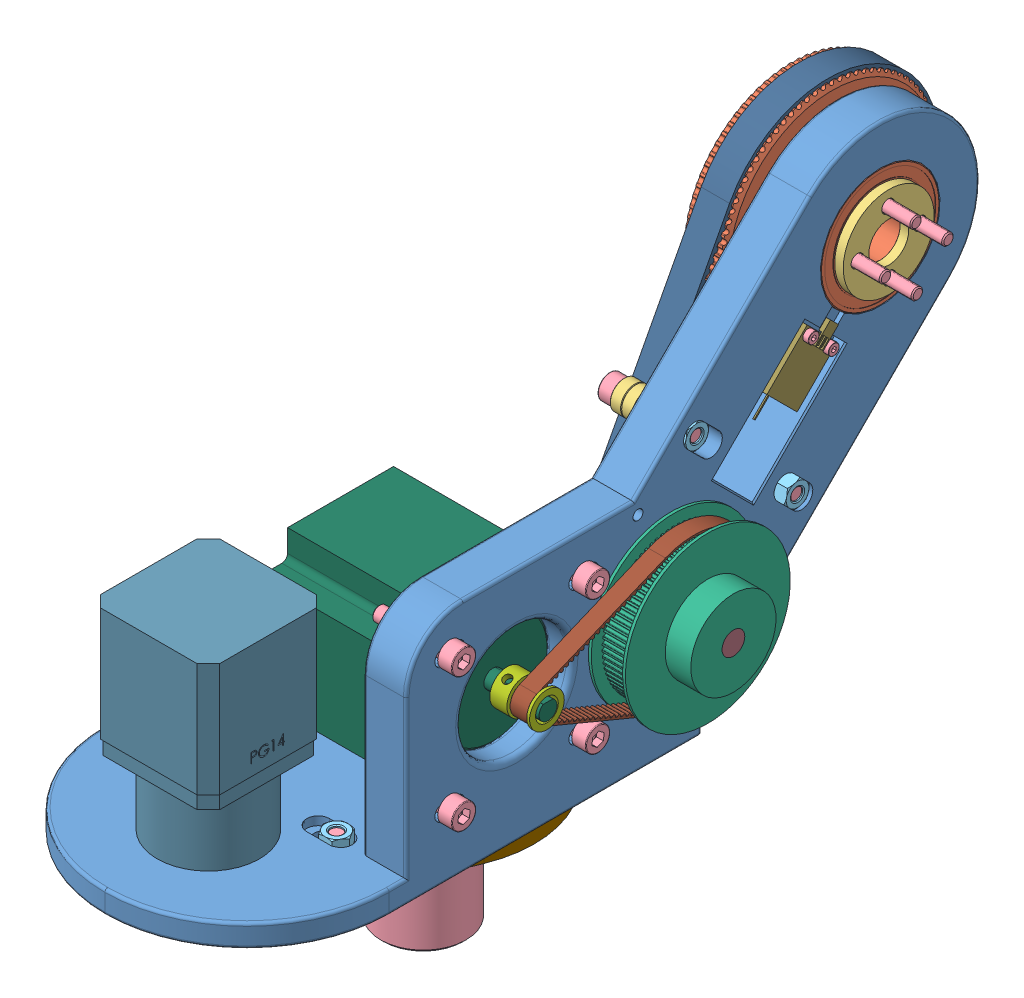
SolidWorks assembly arm1 - Copy, configuration Default. Lengths in mm.
Overall size (123.1 232.46 277.96).
84 component instances, 27 part files, 181 mates.
Components (placement in the parent):
- arm1-1: arm1 [Default] at (0 22.25 32) x (0 0 1) z (0 1 0) size (257.74 100 155.28)
- PulleyHtd3m80Tbore8-2: PulleyHtd3m80Tbore8 [Default] at (25.5 142.4912 -110.7437) x (0 -0.999796 -0.020218) z (1 0 0) size (75.96 75.93 32)
- bearingCover-1: bearingCover [Default] at (50 142.4912 -110.7437) x (0 -0.999796 -0.020218) z (1 0 0) size (32 32 3)
- shaftJ1-1: shaftJ1 [Default] at (0 -34.75 0) x (0 0 -1) z (1 0 0) size (50 69 50)
- Pulleyhtd3m20Tbore8-1: Pulleyhtd3m20Tbore8 [Default] at (0 12.5 75.6) x (1 0 0) z (0 -1 0) size (22 22 24)
- pulley2GT80T-1: pulley2GT80T [Default] at (57.6 67.75 -36.0025) x (0 -0.778145 -0.628085) z (1 0 0) size (58 58 22)
- pulley2GT16Tbore6.35-1: pulley2GT16Tbore6.35 [Default] at (56.1 67.75 17.0975) x (0 0.483708 -0.87523) z (1 0 0) size (12.2 12.2 14)
- PulleyHTD3m15Tbore8-1: PulleyHTD3m15Tbore8 [Default] at (26.5 67.75 -36.0025) x (0 0.57686 0.816843) z (1 0 0) size (14 14 19.5)
- BeltHTD3m312L20T80T-1: BeltHTD3m312L20T80T [Default] at (0 12.5 0) x (0 0 1) z (0 1 0) size (125.04 78.09 10)
- BeltHTD3m363L15T80T-1: BeltHTD3m363L15T80T [Default] at (26.5 142.4912 -110.7437) x (0 -0.707107 0.707107) z (-1 0 0) size (152.76 78.09 10)
- belt2GT210L-1: belt2GT210L [Default] at (56.1 67.75 17.0975) x (0 0 -1) z (1 0 0) size (84.41 51.68 6)
- MagneticSensorV2-2: MagneticSensorV2 [Default] at (45.9 115.6211 -83.8737) x (0 -0.707107 0.707107) z (1 0 0) size (31 15 9)
- shaft8x70-1: shaft8x70 [Default] at (73.1 67.75 -36.0025) x (0 0 1) z (-1 0 0) size (8 8 61)
- Nema17L40PG14-1: Nema17L40PG14 [Default] at (0 99.75 75.6) x (0 0 -1) z (0 -1 0) size (42 42 88.5)
- Nema23_57x57x56-2: Nema23_57x57x56 [Default] at (-12 67.75 17.0975) x (0 0 -1) z (1 0 0) size (57 57 73)
- BeltTensionSpacer-1: BeltTensionSpacer [Default] at (35 113.7119 -46.6091) x (0 -0.41678 -0.909008) z (-1 0 0) size (6.4 6.4 3)
- BeltTensionSpacer-2: BeltTensionSpacer [Default] at (35 78.3566 -81.9645) x (0 -0.41678 -0.909008) z (-1 0 0) size (6.4 6.4 3)
- BeltTensionSpacer-6: BeltTensionSpacer [Default] at (-24.5 19.25 55) x (0.999608 0 0.027999) z (0 1 0) size (6.4 6.4 3)
- BeltTensionSpacer-5: BeltTensionSpacer [Default] at (24.5 22.25 55) x (0.852155 0 0.52329) z (0 -1 0) size (6.4 6.4 3)
- Washer45x60x1-2: Washer45x60x1 [5909K79] at (0 22.25 0) x (0 -1 0) z (0.730209 0 -0.683224) size (1 65 65)
- Washer45x60x1-1: Washer45x60x1 [5909K79] at (0 18.3 0) x (0 -1 0) z (0.528749 0 -0.848778) size (1 65 65)
- NeedleThrustBearing5909_45x60x3-1: NeedleThrustBearing5909_45x60x3 [5909K19] at (0 20.275 0) x (0.862783 0 0.505574) z (0.505574 0 -0.862783) size (65 3 65)
- bearing608 8x22x7-1: bearing608 8x22x7 [Default] at (50 67.75 -36.0025) x (0 -0.065699 -0.997839) z (0 0.997839 -0.065699) size (22 7 22)
- bearing608 8x22x7-2: bearing608 8x22x7 [Default] at (35 67.75 -36.0025) x (0 -0.995759 -0.092005) z (0 -0.092005 0.995759) size (22 7 22)
- bearing6806 30x42x7-3: bearing6806 30x42x7 [5972K282] at (38.5 142.4912 -110.7437) x (0 0.778145 0.628085) z (1 0 0) size (42 42 7)
- bearing6806 30x42x7-4: bearing6806 30x42x7 [5972K282] at (46.5 142.4912 -110.7437) x (0 -0.232241 -0.972658) z (-1 0 0) size (42 42 7)
- Bearing105 5x10x4-1: Bearing105 5x10x4 [7804K106] at (30 113.7119 -46.6091) x (0 0.558787 -0.829311) z (-1 0 0) size (10 10 4)
- Bearing105 5x10x4-4: Bearing105 5x10x4 [7804K106] at (26.1 78.3566 -81.9645) x (0 -0.623411 0.781894) z (-1 0 0) size (10 10 4)
- Bearing105 5x10x4-9: Bearing105 5x10x4 [7804K106] at (24.5 17.25 55) x (0.890608 0 -0.454771) z (0 -1 0) size (10 10 4)
- Bearing105 5x10x4-10: Bearing105 5x10x4 [7804K106] at (24.5 13.25 55) x (0.890608 0 -0.454771) z (0 -1 0) size (10 10 4)
- Bearing105 5x10x4-11: Bearing105 5x10x4 [7804K106] at (-24.5 13.25 55) x (-0.374722 0 0.927137) z (0 1 0) size (10 10 4)
- Bearing105 5x10x4-12: Bearing105 5x10x4 [7804K106] at (-24.5 17.25 55) x (0.156116 0 0.987739) z (0 1 0) size (10 10 4)
- Bearing105 5x10x4-2: Bearing105 5x10x4 [7804K106] at (26 113.7119 -46.6091) x (0 -0.774653 -0.632387) z (-1 0 0) size (10 10 4)
- Bearing105 5x10x4-3: Bearing105 5x10x4 [7804K106] at (30.1 78.3566 -81.9645) x (0 -0.931032 -0.364937) z (1 0 0) size (10 10 4)
- socket head cap screw_iso-13: socket head cap screw_iso [ISO 4762 M4 x 12 - 12N] at (0 38.25 20) x (0 -1 0) z (0 0 1) size (16 7 7)
- socket head cap screw_iso-14: socket head cap screw_iso [ISO 4762 M4 x 12 - 12N] at (20 38.25 0) x (0 -1 0) z (0 0 1) size (16 7 7)
- socket head cap screw_iso-15: socket head cap screw_iso [ISO 4762 M4 x 12 - 12N] at (0 38.25 -20) x (0 -1 0) z (0 0 1) size (16 7 7)
- socket head cap screw_iso-16: socket head cap screw_iso [ISO 4762 M4 x 12 - 12N] at (-20 38.25 0) x (0 -1 0) z (0 0 1) size (16 7 7)
- hex nut style 1 gradeab_iso-1: hex nut style 1 gradeab_iso [ISO - 4032 - M5 - W - N] at (49.7 113.7119 -46.6091) x (0 -0.707107 0.707107) z (1 0 0) size (8 9.24 4.7)
- hex nut style 1 gradeab_iso-2: hex nut style 1 gradeab_iso [ISO - 4032 - M5 - W - N] at (49.7 78.3566 -81.9645) x (0 0.965926 0.258819) z (1 0 0) size (8 9.24 4.7)
- socket head cap screw_iso-20: socket head cap screw_iso [ISO 4762 M5 x 25 - 25N] at (19 113.7119 -46.6091) size (30 8.5 8.5)
- socket head cap screw_iso-21: socket head cap screw_iso [ISO 4762 M5 x 25 - 25N] at (19.1 78.3566 -81.9645) size (30 8.5 8.5)
- socket head cap screw_iso-57: socket head cap screw_iso [ISO 4762 M5 x 20 - 20N] at (24.5 6.25 55) x (0 1 0) z (0 0 1) size (25 8.5 8.5)
- socket head cap screw_iso-58: socket head cap screw_iso [ISO 4762 M5 x 20 - 20N] at (-24.5 6.25 55) x (0 1 0) z (0 0 1) size (25 8.5 8.5)
- hex nut style 1 gradeab_iso-15: hex nut style 1 gradeab_iso [ISO - 4032 - M5 - W - N] at (-24.5 31.95 55) x (-0.866025 0 0.5) z (0 1 0) size (8 9.24 4.7)
- hex nut style 1 gradeab_iso-16: hex nut style 1 gradeab_iso [ISO - 4032 - M5 - W - N] at (24.5 31.95 55) x (-0.866025 0 -0.5) z (0 1 0) size (8 9.24 4.7)
- socket head cap screw_iso-63: socket head cap screw_iso [ISO 4762 M4 x 40 - 20N] at (19 153.4889 -110.5213) size (44 7 7)
- socket head cap screw_iso-64: socket head cap screw_iso [ISO 4762 M4 x 40 - 20N] at (19 142.7136 -121.7415) size (44 7 7)
- socket head cap screw_iso-65: socket head cap screw_iso [ISO 4762 M4 x 40 - 20N] at (19 131.4934 -110.9661) size (44 7 7)
- socket head cap screw_iso-66: socket head cap screw_iso [ISO 4762 M4 x 40 - 20N] at (19 142.2688 -99.746) size (44 7 7)
- socket head cap screw_iso-80: socket head cap screw_iso [ISO 4762 M2 x 12 - 12N] at (51.4 117.7424 -93.066) x (-1 0 0) z (0 0.924225 0.381849) size (14 3.8 3.8)
- socket head cap screw_iso-81: socket head cap screw_iso [ISO 4762 M2 x 12 - 12N] at (51.4 124.8135 -85.995) x (-1 0 0) z (0 0.924225 0.381849) size (14 3.8 3.8)
- hex nut style 1 gradeab_iso-25: hex nut style 1 gradeab_iso [ISO - 4032 - M2 - W - N] at (37.4 117.7424 -93.066) x (0 0 1) z (-1 0 0) size (4 4.62 1.6)
- hex nut style 1 gradeab_iso-26: hex nut style 1 gradeab_iso [ISO - 4032 - M2 - W - N] at (37.4 124.8135 -85.995) x (0 0 1) z (-1 0 0) size (4 4.62 1.6)
- socket head cap screw_iso-96: socket head cap screw_iso [ISO 4762 M5 x 25 - 25N] at (55 91.32 40.6675) x (-1 0 0) z (0 -0.924225 -0.381849) size (30 8.5 8.5)
- socket head cap screw_iso-97: socket head cap screw_iso [ISO 4762 M5 x 25 - 25N] at (55 91.32 -6.4725) x (-1 0 0) z (0 -0.924225 -0.381849) size (30 8.5 8.5)
- socket head cap screw_iso-98: socket head cap screw_iso [ISO 4762 M5 x 25 - 25N] at (55 44.18 -6.4725) x (-1 0 0) z (0 -0.924225 -0.381849) size (30 8.5 8.5)
- socket head cap screw_iso-99: socket head cap screw_iso [ISO 4762 M5 x 25 - 25N] at (55 44.18 40.6675) x (-1 0 0) z (0 -0.924225 -0.381849) size (30 8.5 8.5)
- socket head cap screw_iso-104: socket head cap screw_iso [ISO 4762 M3 x 12 - 12N] at (9.8995 19.25 85.4995) x (0 1 0) z (0 0 1) size (15 5.5 5.5)
- socket head cap screw_iso-105: socket head cap screw_iso [ISO 4762 M3 x 12 - 12N] at (9.8995 19.25 65.7005) x (0 1 0) z (0 0 1) size (15 5.5 5.5)
- socket head cap screw_iso-106: socket head cap screw_iso [ISO 4762 M3 x 12 - 12N] at (-9.8995 19.25 85.4995) x (0 1 0) z (0 0 1) size (15 5.5 5.5)
- socket head cap screw_iso-107: socket head cap screw_iso [ISO 4762 M3 x 12 - 12N] at (-9.8995 19.25 65.7005) x (0 1 0) z (0 0 1) size (15 5.5 5.5)
- hex nut style 1 gradeab_iso-35: hex nut style 1 gradeab_iso [ISO - 4032 - M5 - W - N] at (30.3 91.32 40.6675) x (0 0 1) z (-1 0 0) size (8 9.24 4.7)
- hex nut style 1 gradeab_iso-36: hex nut style 1 gradeab_iso [ISO - 4032 - M5 - W - N] at (30.3 91.32 -6.4725) x (0 0 1) z (-1 0 0) size (8 9.24 4.7)
- hex nut style 1 gradeab_iso-37: hex nut style 1 gradeab_iso [ISO - 4032 - M5 - W - N] at (30.3 44.18 -6.4725) x (0 0 1) z (-1 0 0) size (8 9.24 4.7)
- hex nut style 1 gradeab_iso-38: hex nut style 1 gradeab_iso [ISO - 4032 - M5 - W - N] at (40.3966 44.18 40.6675) x (0 0 -1) z (1 0 0) size (8 9.24 4.7)
- base-1: base [Default] x (1 0 0) z (0 1 0) size (75 138.93 61) (hidden)
- bearing6806 30x42x7-1: bearing6806 30x42x7 [5972K282] at (0 -30.5984 0) x (0.837169 0 0.546944) z (0 -1 0) size (42 42 7) (hidden)
- pulleyHTD3m80Tbase-1: pulleyHTD3m80Tbase [Default] at (0 12 0) x (1 0 0) z (0 1 0) size (75.63 75.63 12) (hidden)
- bearing6806 30x42x7-2: bearing6806 30x42x7 [5972K282] at (0 14.3 0) x (0.999895 0 -0.014508) z (0 1 0) size (42 42 7) (hidden)
- shaftJ1endPlate-1: shaftJ1endPlate [Default] at (0 -34.75 0) x (0 0 -1) z (0 -1 0) size (40 40 6) (hidden)
- MagneticSensor-3: MagneticSensor [Default] at (31.5 -49.5984 0) x (1 0 0) z (0 1 0) size (31 15 7.5) (hidden)
- socket head cap screw_iso-132: socket head cap screw_iso [ISO 4762 M5 x 16 - 16N] at (21 -5 -21) x (0 1 0) z (0 0 1) size (21 8.5 8.5) (hidden)
- socket head cap screw_iso-133: socket head cap screw_iso [ISO 4762 M5 x 16 - 16N] at (21 -5 21) x (0 1 0) z (0 0 1) size (21 8.5 8.5) (hidden)
- socket head cap screw_iso-134: socket head cap screw_iso [ISO 4762 M5 x 16 - 16N] at (-21 -5 21) x (0 1 0) z (0 0 1) size (21 8.5 8.5) (hidden)
- socket head cap screw_iso-135: socket head cap screw_iso [ISO 4762 M5 x 16 - 16N] at (-21 -5 -21) x (0 1 0) z (0 0 1) size (21 8.5 8.5) (hidden)
- socket head cap screw_iso-136: socket head cap screw_iso [ISO 4762 M3 x 16 - 16N] at (12.5 -43.75 0) x (0 1 0) z (0 0 1) size (19 5.5 5.5) (hidden)
- socket head cap screw_iso-137: socket head cap screw_iso [ISO 4762 M3 x 16 - 16N] at (0 -43.75 12.5) x (0 1 0) z (0 0 1) size (19 5.5 5.5) (hidden)
- socket head cap screw_iso-138: socket head cap screw_iso [ISO 4762 M3 x 16 - 16N] at (-12.5 -43.75 0) x (0 1 0) z (0 0 1) size (19 5.5 5.5) (hidden)
- socket head cap screw_iso-139: socket head cap screw_iso [ISO 4762 M3 x 16 - 16N] at (0 -43.75 -12.5) x (0 1 0) z (0 0 1) size (19 5.5 5.5) (hidden)
- socket head cap screw_iso-140: socket head cap screw_iso [ISO 4762 M2 x 12 - 12N] at (23.5 -51.5984 -5) x (0 1 0) z (-0.11823 0 0.992986) size (14 3.8 3.8) (hidden)
- socket head cap screw_iso-141: socket head cap screw_iso [ISO 4762 M2 x 12 - 12N] at (23.5 -51.5984 5) x (0 1 0) z (0 0 1) size (14 3.8 3.8) (hidden)
- hex nut style 1 gradeab_iso-59: hex nut style 1 gradeab_iso [ISO - 4032 - M2 - W - N] at (23.5 -40.9984 -5) x (1 0 0) z (0 1 0) size (4 4.62 1.6) (hidden)
- hex nut style 1 gradeab_iso-60: hex nut style 1 gradeab_iso [ISO - 4032 - M2 - W - N] at (23.5 -40.9984 5) x (1 0 0) z (0 1 0) size (4 4.62 1.6) (hidden)
Mates (geometry in assembly coordinates):
- Fix J1: parallel aligned: plane of base-1 through (37.5 6 37.5) normal (1 0 0); plane of arm1-1 through (50 30.25 -48) normal (1 0 0)
- Concentric1: concentric aligned: cylinder of base-1 through (0 29.44 0) axis (0 -1 0) radius 21.05; cylinder of bearing6806 30x42x7-1 through (0 -34.0984 0) axis (0 -1 0) radius 21
- Coincident1: coincident anti-aligned: plane of base-1 through (0 -34.0984 0) normal (0 1 0); plane of bearing6806 30x42x7-1 through (-11.2944 -34.0984 17.2875) normal (0 -1 0)
- Concentric2: concentric anti-aligned: cylinder of base-1 through (0 6 0) axis (0 -1 0) radius 16; cylinder of pulleyHTD3m80Tbase-1 through (0 10.8 0) axis (0 1 0) radius 21.05
- Concentric3: concentric anti-aligned: cylinder of base-1 through (21 6 21) axis (0 -1 0) radius 2.75; cylinder of pulleyHTD3m80Tbase-1 through (21 6 21) axis (0 1 0) radius 3
- Coincident2: coincident anti-aligned: plane of base-1 through (0 6 0) normal (0 1 0); plane of pulleyHTD3m80Tbase-1 through (0 6 0) normal (0 -1 0)
- Concentric4: concentric aligned: cylinder of base-1 through (21 6 -21) axis (0 -1 0) radius 2.75; cylinder of socket head cap screw_iso-1 through (21 -36.75 -21) axis (0 -1 0) radius 4.25
- Coincident3: coincident anti-aligned: plane of base-1 through (0 0 0) normal (0 -1 0); plane of socket head cap screw_iso-1 through (16.75 0 -21) normal (0 1 0)
- Concentric5: concentric aligned: cylinder of base-1 through (21 6 21) axis (0 -1 0) radius 2.75; cylinder of socket head cap screw_iso-2 through (21 -36.75 21) axis (0 -1 0) radius 4.25
- Coincident4: coincident anti-aligned: plane of base-1 through (0 0 0) normal (0 -1 0); plane of socket head cap screw_iso-2 through (16.75 0 21) normal (0 1 0)
- Concentric6: concentric aligned: cylinder of base-1 through (-21 6 21) axis (0 -1 0) radius 2.75; cylinder of socket head cap screw_iso-3 through (-21 -36.75 21) axis (0 -1 0) radius 4.25
- Coincident5: coincident anti-aligned: plane of base-1 through (0 0 0) normal (0 -1 0); plane of socket head cap screw_iso-3 through (-25.25 0 21) normal (0 1 0)
- Concentric7: concentric aligned: cylinder of base-1 through (-21 6 -21) axis (0 -1 0) radius 2.75; cylinder of socket head cap screw_iso-4 through (-21 -36.75 -21) axis (0 -1 0) radius 4.25
- Coincident6: coincident anti-aligned: plane of base-1 through (0 0 0) normal (0 -1 0); plane of socket head cap screw_iso-4 through (-25.25 0 -21) normal (0 1 0)
- Concentric8: concentric aligned: cylinder of pulleyHTD3m80Tbase-1 through (0 10.8 0) axis (0 1 0) radius 21.05; cylinder of bearing6806 30x42x7-2 through (0 17.8 0) axis (0 1 0) radius 21
- Coincident7: coincident anti-aligned: plane of pulleyHTD3m80Tbase-1 through (0 10.8 0) normal (0 1 0); plane of bearing6806 30x42x7-2 through (-0.2996 10.8 -20.6478) normal (0 -1 0)
- Concentric9: concentric aligned: cylinder of pulleyHTD3m80Tbase-1 through (0 10.8 0) axis (0 1 0) radius 21.05; cylinder of Washer45x60x1-1 through (0 17.8 0) axis (0 1 0) radius 32.5
- Coincident8: coincident anti-aligned: plane of pulleyHTD3m80Tbase-1 through (0 17.8 0) normal (0 1 0); plane of Washer45x60x1-1 through (0 17.8 0) normal (0 -1 0)
- Concentric10: concentric anti-aligned: cylinder of pulleyHTD3m80Tbase-1 through (0 10.8 0) axis (0 1 0) radius 21.05; cylinder of NeedleThrustBearing5909_45x60x3-1 through (0 18.775 0) axis (0 -1 0) radius 32.5
- Distance1: distance = 0.2 mm anti-aligned: plane of NeedleThrustBearing5909_45x60x3-1 through (-16.4311 19 28.0405) normal (0 -1 0); plane of Washer45x60x1-1 through (0 18.8 0) normal (0 1 0)
- Concentric11: concentric aligned: cylinder of pulleyHTD3m80Tbase-1 through (0 10.8 0) axis (0 1 0) radius 21.05; cylinder of Washer45x60x1-2 through (0 21.75 0) axis (0 1 0) radius 22.525
- Distance2: distance = 0.2 mm anti-aligned: plane of NeedleThrustBearing5909_45x60x3-1 through (-16.2626 21.55 27.7529) normal (0 1 0); plane of Washer45x60x1-2 through (0 21.75 0) normal (0 -1 0)
- Concentric12: concentric aligned: cylinder of base-1 through (0 6 0) axis (0 -1 0) radius 16; cylinder of arm1-1 through (0 30.25 0) axis (0 -1 0) radius 15.5
- Coincident12: coincident anti-aligned: plane of arm1-1 through (0 22.75 0) normal (0 -1 0); plane of Washer45x60x1-2 through (0 22.75 0) normal (0 1 0)
- Concentric15: concentric anti-aligned: cylinder of arm1-1 through (0 30.25 75.6) axis (0 -1 0) radius 11.5; cylinder of Nema17L40PG14-1 through (0 30.25 75.6) axis (0 1 0) radius 18
- Concentric16: concentric aligned: cylinder of arm1-1 through (-9.8995 30.25 85.4995) axis (0 -1 0) radius 1.65; cylinder of Nema17L40PG14-1 through (-9.8995 38.25 85.4995) axis (0 -1 0) radius 2
- Coincident16: coincident anti-aligned: plane of arm1-1 through (0 30.25 32) normal (0 1 0); plane of Nema17L40PG14-1 through (0 30.25 75.6) normal (0 -1 0)
- Concentric20: concentric anti-aligned: cylinder of Nema17L40PG14-1 through (0 11.25 75.6) axis (0 1 0) radius 4; cylinder of Pulleyhtd3m20Tbore8-1 through (0 30 75.6) axis (0 -1 0) radius 11
- Coincident17: coincident anti-aligned: plane of pulleyHTD3m80Tbase-1 through (0 18 0) normal (0 1 0); plane of Pulleyhtd3m20Tbore8-1 through (0 18 75.6) normal (0 -1 0)
- Concentric21: concentric aligned: cylinder of NeedleThrustBearing5909_45x60x3-1 through (0 18.775 0) axis (0 -1 0) radius 32.5; cylinder of BeltHTD3m312L20T80T-1 through (0 17.5 0) axis (0 -1 0) radius 39.0462
- Concentric22: concentric aligned: cylinder of Pulleyhtd3m20Tbore8-1 through (0 30 75.6) axis (0 -1 0) radius 11; cylinder of BeltHTD3m312L20T80T-1 through (0 17.5 75.6) axis (0 -1 0) radius 10.3983
- Distance3: distance = 0.5 mm anti-aligned: plane of Pulleyhtd3m20T-1 through (0 18 75.6) normal (0 -1 0); plane of BeltHTD3m312L20T80T-1 through (0 17.5 0) normal (0 1 0)
- Concentric23: concentric aligned: cylinder of arm1-1 through (0 30.25 0) axis (0 -1 0) radius 15.5; cylinder of shaftJ1-1 through (0 30.25 0) axis (0 -1 0) radius 15
- Concentric24: concentric aligned: cylinder of arm1-1 through (0 30.25 20) axis (0 -1 0) radius 2.75; cylinder of shaftJ1-1 through (0 34.25 20) axis (0 -1 0) radius 2.25
- Coincident19: coincident anti-aligned: plane of arm1-1 through (0 30.25 32) normal (0 1 0); plane of shaftJ1-1 through (0 30.25 0) normal (0 -1 0)
- Coincident24: coincident anti-aligned: plane of shaftJ1-1 through (0 -34.75 0) normal (0 -1 0); plane of shaftJ1endPlate-1 through (0 -34.75 0) normal (0 1 0)
- Concentric29: concentric anti-aligned: cylinder of shaftJ1-1 through (0 -14.75 12.5) axis (0 -1 0) radius 1.4; cylinder of shaftJ1endPlate-1 through (0 -40.75 12.5) axis (0 1 0) radius 1.75
- Concentric36: concentric anti-aligned: cylinder of shaftJ1-1 through (0 34.25 20) axis (0 -1 0) radius 2.25; cylinder of socket head cap screw_iso1-13 through (0 70 20) axis (0 1 0) radius 3.5
- Coincident31: coincident anti-aligned: plane of shaftJ1-1 through (0 34.25 0) normal (0 1 0); plane of socket head cap screw_iso1-13 through (3.5 34.25 20) normal (0 -1 0)
- Concentric37: concentric anti-aligned: cylinder of shaftJ1-1 through (20 34.25 0) axis (0 -1 0) radius 2.25; cylinder of socket head cap screw_iso1-14 through (20 70 0) axis (0 1 0) radius 3.5
- Coincident32: coincident anti-aligned: plane of shaftJ1-1 through (0 34.25 0) normal (0 1 0); plane of socket head cap screw_iso1-14 through (23.5 34.25 0) normal (0 -1 0)
- Concentric38: concentric anti-aligned: cylinder of shaftJ1-1 through (0 34.25 -20) axis (0 -1 0) radius 2.25; cylinder of socket head cap screw_iso1-15 through (0 70 -20) axis (0 1 0) radius 3.5
- Coincident33: coincident anti-aligned: plane of shaftJ1-1 through (0 34.25 0) normal (0 1 0); plane of socket head cap screw_iso1-15 through (3.5 34.25 -20) normal (0 -1 0)
- Concentric39: concentric anti-aligned: cylinder of shaftJ1-1 through (-20 34.25 0) axis (0 -1 0) radius 2.25; cylinder of socket head cap screw_iso1-16 through (-20 70 0) axis (0 1 0) radius 3.5
- Coincident34: coincident anti-aligned: circle of shaftJ1-1; plane of socket head cap screw_iso1-16 through (-16.5 34.25 0) normal (0 -1 0)
- Concentric41: concentric anti-aligned: cylinder of arm1-1 through (35 67.75 17.0975) axis (1 0 0) radius 19.5; cylinder of Nema23_57x57x56-2 through (61 67.75 17.0975) axis (-1 0 0) radius 3.175
- Coincident36: coincident anti-aligned: plane of arm1-1 through (40 22.25 32) normal (-1 0 0); plane of Nema23_57x57x56-2 through (40 67.75 17.0975) normal (1 0 0)
- Parallel2: parallel aligned: plane of arm1-1 through (35 105.25 55.9949) normal (0 1 0); plane of Nema23_57x57x56-2 through (40 96.25 45.5975) normal (0 1 0)
- Concentric42: concentric anti-aligned: cylinder of pulley2GT16Tbore6.35-1 through (46.6 67.75 17.0975) axis (1 0 0) radius 6.1; cylinder of Nema23_57x57x56-2 through (61 67.75 17.0975) axis (-1 0 0) radius 3.175
- Concentric43: concentric aligned: cylinder of arm1-1 through (43 67.75 -36.0025) axis (1 0 0) radius 11.05; cylinder of bearing608 8x22x7-1 through (43 67.75 -36.0025) axis (1 0 0) radius 11
- Coincident41: coincident anti-aligned: plane of arm1-1 through (43 67.75 -36.0025) normal (1 0 0); plane of bearing608 8x22x7-1 through (43 67.75 -36.0025) normal (-1 0 0)
- Concentric44: concentric aligned: cylinder of arm1-1 through (42 67.75 -36.0025) axis (-1 0 0) radius 11.05; cylinder of bearing608 8x22x7-2 through (42 67.75 -36.0025) axis (-1 0 0) radius 11
- Coincident42: coincident anti-aligned: plane of arm1-1 through (42 67.75 -36.0025) normal (-1 0 0); plane of bearing608 8x22x7-2 through (42 67.75 -36.0025) normal (1 0 0)
- Concentric45: concentric anti-aligned: cylinder of arm1-1 through (43 142.4912 -110.7437) axis (1 0 0) radius 21.05; cylinder of bearing6806 30x42x7-4 through (43 142.4912 -110.7437) axis (-1 0 0) radius 21
- Coincident43: coincident anti-aligned: plane of arm1-1 through (43 142.4912 -110.7437) normal (1 0 0); plane of bearing6806 30x42x7-4 through (43 122.4058 -105.9479) normal (-1 0 0)
- Concentric46: concentric anti-aligned: cylinder of arm1-1 through (42 142.4912 -110.7437) axis (-1 0 0) radius 21.05; cylinder of bearing6806 30x42x7-3 through (42 142.4912 -110.7437) axis (1 0 0) radius 21
- Coincident44: coincident anti-aligned: plane of arm1-1 through (42 142.4912 -110.7437) normal (-1 0 0); plane of bearing6806 30x42x7-3 through (42 129.5212 -94.675) normal (1 0 0)
- Concentric47: concentric aligned: cylinder of bearing608 8x22x7-1 through (43 67.75 -36.0025) axis (1 0 0) radius 4; cylinder of pulley2GT80T-1 through (51.1 67.75 -36.0025) axis (1 0 0) radius 4
- Distance4: distance = 0.5 mm aligned: plane of pulley2GT16Tbore6.35-1 through (52.6 67.75 17.0975) normal (1 0 0); plane of pulley2GT80Tbore8-1 through (52.1 67.75 -36.0025) normal (1 0 0)
- Concentric48: concentric anti-aligned: cylinder of bearing608 8x22x7-2 through (42 67.75 -36.0025) axis (-1 0 0) radius 4; cylinder of shaft8x70-1 through (12.1 67.75 -36.0025) axis (1 0 0) radius 4
- Coincident46: coincident aligned: plane of pulley2GT80T-1 through (73.1 67.75 -36.0025) normal (1 0 0); plane of shaft8x70-1 through (73.1 67.75 -36.0025) normal (1 0 0)
- disPulley1J1: distance = 5 mm anti-aligned: plane of pulley2GT16Tbore6.35-1 through (46.6 67.75 17.0975) normal (-1 0 0); plane of Nema23_57x57x56-2 through (41.6 67.75 17.0975) normal (1 0 0)
- Concentric51: concentric aligned: cylinder of pulley2GT80T-1 through (73.1 67.75 -36.0025) axis (-1 0 0) radius 15; cylinder of belt2GT210L-1 through (59.1 67.75 -36.0025) axis (-1 0 0) radius 25.84
- Concentric52: concentric anti-aligned: cylinder of pulley2GT16Tbore6.35-1 through (46.6 67.75 17.0975) axis (1 0 0) radius 6.1; cylinder of belt2GT210L-1 through (59.1 67.75 17.0975) axis (-1 0 0) radius 5.47
- Distance6: distance = 0.5 mm anti-aligned: plane of pulley2GT16Tbore6.35-1 through (52.6 67.75 17.0975) normal (1 0 0); plane of belt2GT210L-1 through (53.1 67.75 -36.0025) normal (-1 0 0)
- Concentric58: concentric aligned: cylinder of arm1-1 through (35 113.7119 -46.6091) axis (1 0 0) radius 2.75; cylinder of hex nut style 1 gradeab_isoV1-1 through (24.6625 113.7119 -46.6091) axis (1 0 0) radius 2.5
- Coincident53: coincident anti-aligned: plane of arm1-1 through (45 114.7726 -45.5485) normal (1 0 0); plane of hex nut style 1 gradeab_isoV1-1 through (45 119.3688 -52.266) normal (-1 0 0)
- Coincident54: coincident anti-aligned: plane of arm1-1 through (45 117.601 -48.3769) normal (0 -0.707107 0.707107); plane of hex nut style 1 gradeab_isoV1-1 through (45 114.9074 -51.0705) normal (0 0.707107 -0.707107)
- Concentric591: concentric aligned: cylinder of arm1-1 through (35 78.3566 -81.9645) axis (1 0 0) radius 2.75; cylinder of hex nut style 1 gradeab_isoV1-2 through (24.6625 78.3566 -81.9645) axis (1 0 0) radius 2.5
- Coincident551: coincident anti-aligned: plane of arm1-1 through (45 82.9528 -77.3683) normal (1 0 0); plane of hex nut style 1 gradeab_isoV1-2 through (45 70.6292 -84.035) normal (-1 0 0)
- Coincident56: coincident anti-aligned: plane of arm1-1 through (45 85.7812 -80.1967) normal (0 -0.707107 0.707107); plane of hex nut style 1 gradeab_isoV1-2 through (45 79.552 -86.4259) normal (0 0.707107 -0.707107)
- Concentric60: concentric anti-aligned: cylinder of arm1-1 through (35 113.7119 -46.6091) axis (1 0 0) radius 2.75; cylinder of Bearing105 5x10x4-1 through (28 113.7119 -46.6091) axis (-1 0 0) radius 5
- Distance8: distance = 3 mm anti-aligned: plane of arm1-1 through (35 142.4912 -110.7437) normal (-1 0 0); plane of Bearing105 5x10x4-1 through (32 109.7312 -49.2913) normal (1 0 0)
- Concentric61: concentric aligned: cylinder of Bearing105 5x10x4-1 through (28 113.7119 -46.6091) axis (-1 0 0) radius 5; cylinder of Bearing105 5x10x4-2 through (24 113.7119 -46.6091) axis (-1 0 0) radius 5
- Coincident58: coincident anti-aligned: plane of Bearing105 5x10x4-1 through (28 109.7312 -49.2913) normal (-1 0 0); plane of Bearing105 5x10x4-2 through (28 110.6765 -42.8908) normal (1 0 0)
- Concentric63: concentric aligned: cylinder of Bearing105 5x10x4-2 through (24 113.7119 -46.6091) axis (-1 0 0) radius 3.4863; cylinder of socket head cap screw_iso1-20 through (-12.75 113.7119 -46.6091) axis (-1 0 0) radius 4.25
- Coincident60: coincident anti-aligned: plane of Bearing105 5x10x4-2 through (24 111.5073 -43.9085) normal (-1 0 0); plane of socket head cap screw_iso1-20 through (24 117.9619 -46.6091) normal (1 0 0)
- Concentric64: concentric anti-aligned: cylinder of socket head cap screw_iso1-20 through (-12.75 113.7119 -46.6091) axis (-1 0 0) radius 2.5; cylinder of BeltTensionSpacer-1 through (32 113.7119 -46.6091) axis (1 0 0) radius 3.2
- Coincident61: coincident anti-aligned: plane of arm1-1 through (35 142.4912 -110.7437) normal (-1 0 0); plane of BeltTensionSpacer-1 through (35 113.7119 -46.6091) normal (1 0 0)
- Concentric65: concentric aligned: cylinder of arm1-1 through (35 78.3566 -81.9645) axis (1 0 0) radius 2.75; cylinder of BeltTensionSpacer-2 through (32 78.3566 -81.9645) axis (1 0 0) radius 3.2
- Coincident62: coincident aligned: plane of arm1-1 through (35 142.4912 -110.7437) normal (-1 0 0); circle of BeltTensionSpacer-2
- Concentric66: concentric aligned: cylinder of Bearing105 5x10x4-3 through (32.1 78.3566 -81.9645) axis (1 0 0) radius 5; cylinder of BeltTensionSpacer-2 through (32 78.3566 -81.9645) axis (1 0 0) radius 3.2
- Coincident63: coincident anti-aligned: plane of Bearing105 5x10x4-3 through (32 79.8214 -85.7014) normal (1 0 0); plane of BeltTensionSpacer-2 through (32 78.3566 -81.9645) normal (-1 0 0)
- Coincident64: coincident anti-aligned: plane of Bearing105 5x10x4-3 through (28.1 80.1083 -86.4334) normal (-1 0 0); plane of Bearing105 5x10x4-4 through (28.1 82.1097 -78.9721) normal (1 0 0)
- Concentric67: concentric anti-aligned: cylinder of Bearing105 5x10x4-3 through (32.1 78.3566 -81.9645) axis (1 0 0) radius 5; cylinder of Bearing105 5x10x4-4 through (24.1 78.3566 -81.9645) axis (-1 0 0) radius 5
- Concentric681: concentric aligned: cylinder of Bearing105 5x10x4-4 through (24.1 78.3566 -81.9645) axis (-1 0 0) radius 4.0137; cylinder of socket head cap screw_iso1-21 through (-12.65 78.3566 -81.9645) axis (-1 0 0) radius 4.25
- Coincident651: coincident anti-aligned: plane of Bearing105 5x10x4-4 through (24.1 82.1097 -78.9721) normal (-1 0 0); plane of socket head cap screw_iso1-21 through (24.1 82.6066 -81.9645) normal (1 0 0)
- Concentric786: concentric anti-aligned: cylinder of base-1 through (23.5 -46.0984 5) axis (0 1 0) radius 1.25; cylinder of MagneticSensor-3 through (23.5 -42.0984 5) axis (0 -1 0) radius 1.25
- Concentric787: concentric anti-aligned: cylinder of base-1 through (23.5 -46.0984 -5) axis (0 1 0) radius 1.25; cylinder of MagneticSensor-3 through (23.5 -42.0984 -5) axis (0 -1 0) radius 1.25
- Coincident749: coincident anti-aligned: plane of base-1 through (0 -46.0984 0) normal (0 -1 0); plane of MagneticSensor-3 through (31.5 -46.0984 0) normal (0 1 0)
- Coincident751: coincident anti-aligned: plane of arm1-1 through (45.9 22.25 32) normal (1 0 0); plane of MagneticSensorV2-2 through (45.9 115.6211 -83.8737) normal (-1 0 0)
- Concentric790: concentric anti-aligned: cylinder of arm1-1 through (35 117.7424 -93.066) axis (1 0 0) radius 1.25; cylinder of MagneticSensorV2-2 through (50.9 117.7424 -93.066) axis (-1 0 0) radius 1.25
- Concentric791: concentric anti-aligned: cylinder of arm1-1 through (35 124.8135 -85.995) axis (1 0 0) radius 1.25; cylinder of MagneticSensorV2-2 through (50.9 124.8135 -85.995) axis (-1 0 0) radius 1.25
- Concentric7962: concentric aligned: cylinder of shaft8x70-1 through (12.1 67.75 -36.0025) axis (1 0 0) radius 4; cylinder of PulleyHTD3m15Tbore8-1 through (13.5 67.75 -36.0025) axis (1 0 0) radius 7
- Concentric7963: concentric anti-aligned: cylinder of shaftJ1endPlate-1 through (12.5 -40.75 0) axis (0 1 0) radius 1.75; cylinder of socket head cap screw_iso1-136 through (12.5 -75.5 0) axis (0 -1 0) radius 2.75
- Coincident7532: coincident anti-aligned: plane of shaftJ1endPlate-1 through (0 -40.75 0) normal (0 -1 0); plane of socket head cap screw_iso1-136 through (9.75 -40.75 0) normal (0 1 0)
- Concentric7964: concentric anti-aligned: cylinder of shaftJ1endPlate-1 through (0 -40.75 12.5) axis (0 1 0) radius 1.75; cylinder of socket head cap screw_iso1-137 through (0 -75.5 12.5) axis (0 -1 0) radius 2.75
- Coincident7533: coincident anti-aligned: plane of shaftJ1endPlate-1 through (0 -40.75 0) normal (0 -1 0); plane of socket head cap screw_iso1-137 through (-2.75 -40.75 12.5) normal (0 1 0)
- Concentric7965: concentric anti-aligned: cylinder of shaftJ1endPlate-1 through (-12.5 -40.75 0) axis (0 1 0) radius 1.75; cylinder of socket head cap screw_iso1-138 through (-12.5 -75.5 0) axis (0 -1 0) radius 2.75
- Coincident7534: coincident anti-aligned: plane of shaftJ1endPlate-1 through (0 -40.75 0) normal (0 -1 0); plane of socket head cap screw_iso1-138 through (-15.25 -40.75 0) normal (0 1 0)
- Concentric7966: concentric anti-aligned: cylinder of shaftJ1endPlate-1 through (0 -40.75 -12.5) axis (0 1 0) radius 1.75; cylinder of socket head cap screw_iso1-139 through (0 -75.5 -12.5) axis (0 -1 0) radius 2.75
- Coincident7535: coincident anti-aligned: plane of shaftJ1endPlate-1 through (0 -40.75 0) normal (0 -1 0); plane of socket head cap screw_iso1-139 through (-2.75 -40.75 -12.5) normal (0 1 0)
- Concentric7967: concentric aligned: cylinder of shaftJ1-1 through (0 30.25 0) axis (0 -1 0) radius 15; cylinder of shaftJ1endPlate-1 through (0 -35.75 0) axis (0 -1 0) radius 20
- Distance21: distance = 2 mm anti-aligned: plane of PulleyHTD3m15Tbore8-1 through (33 67.75 -36.0025) normal (1 0 0); plane of arm1-1 through (35 142.4912 -110.7437) normal (-1 0 0)
- Distance22: distance = 0.5 mm anti-aligned: plane of PulleyHTD3m15Tbore8-1 through (21 67.75 -36.0025) normal (1 0 0); plane of BeltHTD3m363L15T80T-1 through (21.5 142.4912 -110.7437) normal (-1 0 0)
- Concentric7968: concentric anti-aligned: cylinder of arm1-1 through (35 142.4912 -110.7437) axis (1 0 0) radius 35; cylinder of PulleyHtd3m80Tbore8-2 through (50 142.4912 -110.7437) axis (-1 0 0) radius 15
- Coincident7539: coincident anti-aligned: plane of arm1-1 through (35 142.4912 -110.7437) normal (-1 0 0); plane of PulleyHtd3m80Tbore8-2 through (35 142.4912 -110.7437) normal (1 0 0)
- Concentric7969: concentric anti-aligned: cylinder of PulleyHtd3m80Tbore8-2 through (18 142.4912 -110.7437) axis (1 0 0) radius 7; cylinder of bearingCover-1 through (53 142.4912 -110.7437) axis (-1 0 0) radius 7
- Coincident7540: coincident anti-aligned: plane of PulleyHtd3m80Tbore8-2 through (50 142.4912 -110.7437) normal (1 0 0); plane of bearingCover-1 through (50 142.4912 -110.7437) normal (-1 0 0)
- Concentric7970: concentric anti-aligned: cylinder of PulleyHtd3m80Tbore8-2 through (18 131.4934 -110.9661) axis (1 0 0) radius 2.25; cylinder of bearingCover-1 through (53 131.4934 -110.9661) axis (-1 0 0) radius 2.25
- Concentric7973: concentric aligned: cylinder of BeltHTD3m363L15T80T-1 through (21.5 142.4912 -110.7437) axis (1 0 0) radius 39.0462; cylinder of PulleyHtd3m80Tbore8-2 through (18 142.4912 -110.7437) axis (1 0 0) radius 7
- Concentric7974: concentric aligned: cylinder of shaft8x70-1 through (12.1 67.75 -36.0025) axis (1 0 0) radius 4; cylinder of BeltHTD3m363L15T80T-1 through (21.5 67.75 -36.0025) axis (1 0 0) radius 8.011
- Concentric7985: concentric anti-aligned: cylinder of arm1-1 through (24.5 177.4912 55) axis (0 -1 0) radius 2.75; cylinder of BeltTensionSpacer-5 through (24.5 19.25 55) axis (0 1 0) radius 3.2
- Coincident7549: coincident anti-aligned: plane of arm1-1 through (0 22.25 32) normal (0 -1 0); plane of BeltTensionSpacer-5 through (24.5 22.25 55) normal (0 1 0)
- Concentric7986: concentric anti-aligned: cylinder of BeltTensionSpacer-5 through (24.5 19.25 55) axis (0 1 0) radius 3.2; cylinder of Bearing105 5x10x4-9 through (24.5 15.25 55) axis (0 -1 0) radius 5
- Coincident7550: coincident anti-aligned: plane of BeltTensionSpacer-5 through (24.5 19.25 55) normal (0 -1 0); plane of Bearing105 5x10x4-9 through (26.6829 19.25 59.2749) normal (0 1 0)
- Coincident7551: coincident anti-aligned: plane of Bearing105 5x10x4-9 through (26.6829 15.25 59.2749) normal (0 -1 0); plane of Bearing105 5x10x4-10 through (26.6829 15.25 59.2749) normal (0 1 0)
- Concentric7987: concentric aligned: cylinder of Bearing105 5x10x4-9 through (24.5 15.25 55) axis (0 -1 0) radius 5; cylinder of Bearing105 5x10x4-10 through (24.5 11.25 55) axis (0 -1 0) radius 5
- Concentric7988: concentric aligned: cylinder of arm1-1 through (-24.5 177.4912 55) axis (0 -1 0) radius 2.75; cylinder of BeltTensionSpacer-6 through (-24.5 22.25 55) axis (0 -1 0) radius 3.2
- Coincident7552: coincident anti-aligned: plane of arm1-1 through (0 22.25 32) normal (0 -1 0); plane of BeltTensionSpacer-6 through (-24.5 22.25 55) normal (0 1 0)
- Concentric7989: concentric anti-aligned: cylinder of BeltTensionSpacer-6 through (-24.5 22.25 55) axis (0 -1 0) radius 3.2; cylinder of Bearing105 5x10x4-12 through (-24.5 19.25 55) axis (0 1 0) radius 5
- Coincident7553: coincident anti-aligned: plane of BeltTensionSpacer-6 through (-24.5 19.25 55) normal (0 -1 0); plane of Bearing105 5x10x4-12 through (-19.7589 19.25 54.2506) normal (0 1 0)
- Concentric7990: concentric aligned: cylinder of Bearing105 5x10x4-11 through (-24.5 15.25 55) axis (0 1 0) radius 5; cylinder of Bearing105 5x10x4-12 through (-24.5 19.25 55) axis (0 1 0) radius 5
- Coincident7554: coincident anti-aligned: plane of Bearing105 5x10x4-11 through (-20.0497 15.25 56.7987) normal (0 1 0); plane of Bearing105 5x10x4-12 through (-19.7589 15.25 54.2506) normal (0 -1 0)
- Concentric7991: concentric aligned: cylinder of Bearing105 5x10x4-10 through (24.5 11.25 55) axis (0 -1 0) radius 3.4863; cylinder of socket head cap screw_iso1-57 through (24.5 -25.5 55) axis (0 -1 0) radius 4.25
- Coincident7555: coincident anti-aligned: plane of Bearing105 5x10x4-10 through (26.0855 11.25 58.1049) normal (0 -1 0); plane of socket head cap screw_iso1-57 through (20.25 11.25 55) normal (0 1 0)
- Concentric7992: concentric anti-aligned: cylinder of Bearing105 5x10x4-11 through (-24.5 15.25 55) axis (0 1 0) radius 3.4863; cylinder of socket head cap screw_iso1-58 through (-24.5 -25.5 55) axis (0 -1 0) radius 4.25
- Coincident7556: coincident anti-aligned: plane of Bearing105 5x10x4-11 through (-21.9967 11.25 56.0117) normal (0 -1 0); plane of socket head cap screw_iso1-58 through (-28.75 11.25 55) normal (0 1 0)
- Concentric7994: concentric anti-aligned: cylinder of arm1-1 through (-24.5 177.4912 55) axis (0 -1 0) radius 2.75; cylinder of hex nut style 1 gradeab_isoV1-15 through (-24.5 6.9125 55) axis (0 1 0) radius 2.5
- Coincident7558: coincident anti-aligned: plane of arm1-1 through (-26 27.25 55) normal (0 1 0); plane of hex nut style 1 gradeab_isoV1-15 through (-17.5718 27.25 51) normal (0 -1 0)
- Concentric7995: concentric anti-aligned: cylinder of arm1-1 through (24.5 177.4912 55) axis (0 -1 0) radius 2.75; cylinder of hex nut style 1 gradeab_isoV1-16 through (24.5 6.9125 55) axis (0 1 0) radius 2.5
- Coincident7559: coincident anti-aligned: plane of arm1-1 through (18 27.25 55) normal (0 1 0); plane of hex nut style 1 gradeab_isoV1-16 through (31.4282 27.25 59) normal (0 -1 0)
- Coincident7560: coincident anti-aligned: plane of arm1-1 through (18 27.25 51) normal (0 0 1); plane of hex nut style 1 gradeab_isoV1-16 through (26.8094 27.25 51) normal (0 0 -1)
- Coincident7561: coincident anti-aligned: plane of arm1-1 through (-26 27.25 51) normal (0 0 1); plane of hex nut style 1 gradeab_isoV1-15 through (-22.1906 27.25 51) normal (0 0 -1)
- Concentric8000: concentric anti-aligned: cylinder of PulleyHtd3m80Tbore8-2 through (18 153.4889 -110.5213) axis (1 0 0) radius 2.25; cylinder of socket head cap screw_iso1-63 through (-12.75 153.4889 -110.5213) axis (-1 0 0) radius 3.5
- Coincident7570: coincident anti-aligned: plane of PulleyHtd3m80Tbore8-2 through (23 153.4889 -110.5213) normal (-1 0 0); plane of socket head cap screw_iso1-63 through (23 156.9889 -110.5213) normal (1 0 0)
- Concentric8001: concentric anti-aligned: cylinder of PulleyHtd3m80Tbore8-2 through (18 142.7136 -121.7415) axis (1 0 0) radius 2.25; cylinder of socket head cap screw_iso1-64 through (-12.75 142.7136 -121.7415) axis (-1 0 0) radius 3.5
- Coincident7571: coincident anti-aligned: plane of PulleyHtd3m80Tbore8-2 through (23 142.7136 -121.7415) normal (-1 0 0); plane of socket head cap screw_iso1-64 through (23 146.2136 -121.7415) normal (1 0 0)
- Concentric8002: concentric aligned: cylinder of PulleyHtd3m80Tbore8-2 through (23 131.4934 -110.9661) axis (-1 0 0) radius 3.6; cylinder of socket head cap screw_iso1-65 through (-12.75 131.4934 -110.9661) axis (-1 0 0) radius 3.5
- Coincident7572: coincident anti-aligned: plane of PulleyHtd3m80Tbore8-2 through (23 131.4934 -110.9661) normal (-1 0 0); plane of socket head cap screw_iso1-65 through (23 134.9934 -110.9661) normal (1 0 0)
- Concentric8003: concentric anti-aligned: cylinder of PulleyHtd3m80Tbore8-2 through (18 142.2688 -99.746) axis (1 0 0) radius 2.25; cylinder of socket head cap screw_iso1-66 through (-12.75 142.2688 -99.746) axis (-1 0 0) radius 3.5
- Coincident7573: coincident anti-aligned: plane of PulleyHtd3m80Tbore8-2 through (23 142.2688 -99.746) normal (-1 0 0); plane of socket head cap screw_iso1-66 through (23 145.7688 -99.746) normal (1 0 0)
- Concentric8033: concentric anti-aligned: cylinder of MagneticSensorV2-2 through (50.9 117.7424 -93.066) axis (-1 0 0) radius 1.25; cylinder of socket head cap screw_iso1-80 through (83.15 117.7424 -93.066) axis (1 0 0) radius 1.9
- Coincident7610: coincident anti-aligned: plane of MagneticSensorV2-2 through (49.4 115.6211 -83.8737) normal (1 0 0); plane of socket head cap screw_iso1-80 through (49.4 117.0169 -91.31) normal (-1 0 0)
- Concentric8034: concentric anti-aligned: cylinder of MagneticSensorV2-2 through (50.9 124.8135 -85.995) axis (-1 0 0) radius 1.25; cylinder of socket head cap screw_iso1-81 through (83.15 124.8135 -85.995) axis (1 0 0) radius 1.9
- Coincident7611: coincident anti-aligned: plane of MagneticSensorV2-2 through (49.4 115.6211 -83.8737) normal (1 0 0); plane of socket head cap screw_iso1-81 through (49.4 124.088 -84.2389) normal (-1 0 0)
- Concentric8035: concentric aligned: cylinder of MagneticSensor-3 through (23.5 -42.0984 -5) axis (0 -1 0) radius 1.25; cylinder of socket head cap screw_iso-82 through (23.5 -83.3484 -5) axis (0 -1 0) radius 1.9
- Concentric8036: concentric aligned: cylinder of MagneticSensor-3 through (23.5 -42.0984 5) axis (0 -1 0) radius 1.25; cylinder of socket head cap screw_iso-83 through (23.5 -83.3484 5) axis (0 -1 0) radius 1.9
- Coincident7612: coincident anti-aligned: plane of MagneticSensor-3 through (31.5 -49.5984 0) normal (0 -1 0); plane of socket head cap screw_iso-83 through (21.6 -49.5984 5) normal (0 1 0)
- Concentric8037: concentric aligned: cylinder of base-1 through (23.5 -46.0984 -5) axis (0 1 0) radius 1.25; cylinder of hex nut style 1 gradeab_iso-23 through (23.5 -66.0359 -5) axis (0 1 0) radius 1
- Coincident7613: coincident anti-aligned: plane of base-1 through (31 -42.5984 13) normal (0 1 0); plane of hex nut style 1 gradeab_iso-23 through (23.5 -42.5984 -7.3094) normal (0 -1 0)
- Concentric8038: concentric aligned: cylinder of base-1 through (23.5 -46.0984 5) axis (0 1 0) radius 1.25; cylinder of hex nut style 1 gradeab_iso-24 through (23.5 -66.0359 5) axis (0 1 0) radius 1
- Coincident7614: coincident anti-aligned: plane of base-1 through (31 -42.5984 13) normal (0 1 0); plane of hex nut style 1 gradeab_iso-24 through (23.5 -42.5984 2.6906) normal (0 -1 0)
- Concentric8039: concentric anti-aligned: cylinder of arm1-1 through (35 117.7424 -93.066) axis (1 0 0) radius 1.25; cylinder of hex nut style 1 gradeab_isoV1-25 through (62.4375 117.7424 -93.066) axis (-1 0 0) radius 1
- Coincident7615: coincident anti-aligned: plane of arm1-1 through (39 22.25 32) normal (-1 0 0); plane of hex nut style 1 gradeab_isoV1-25 through (39 120.0519 -93.066) normal (1 0 0)
- Concentric8040: concentric anti-aligned: cylinder of arm1-1 through (35 124.8135 -85.995) axis (1 0 0) radius 1.25; cylinder of hex nut style 1 gradeab_isoV1-26 through (62.4375 124.8135 -85.995) axis (-1 0 0) radius 1
- Coincident7616: coincident anti-aligned: plane of arm1-1 through (39 22.25 32) normal (-1 0 0); plane of hex nut style 1 gradeab_isoV1-26 through (39 127.1229 -85.995) normal (1 0 0)
- Concentric8058: concentric aligned: cylinder of Nema23_57x57x56-2 through (-12 91.32 40.6675) axis (1 0 0) radius 2.75; cylinder of socket head cap screw_iso1-96 through (86.75 91.32 40.6675) axis (1 0 0) radius 2.5
- Coincident7633: coincident anti-aligned: plane of arm1-1 through (50 30.25 -48) normal (1 0 0); plane of socket head cap screw_iso1-96 through (50 92.9429 36.7395) normal (-1 0 0)
- Coincident76341: coincident anti-aligned: plane of arm1-1 through (50 30.25 -48) normal (1 0 0); plane of socket head cap screw_iso1-98 through (50 45.8029 -10.4005) normal (-1 0 0)
- Coincident76351: coincident anti-aligned: plane of arm1-1 through (50 30.25 -48) normal (1 0 0); plane of socket head cap screw_iso1-99 through (50 45.8029 36.7395) normal (-1 0 0)
- Concentric8059: concentric aligned: cylinder of Nema23_57x57x56-2 through (-12 44.18 40.6675) axis (1 0 0) radius 2.75; cylinder of socket head cap screw_iso1-99 through (86.75 44.18 40.6675) axis (1 0 0) radius 4.25
- Concentric8060: concentric aligned: cylinder of Nema23_57x57x56-2 through (-12 44.18 -6.4725) axis (1 0 0) radius 2.75; circle of socket head cap screw_iso-98
- Concentric8061: concentric aligned: cylinder of Nema23_57x57x56-2 through (-12 91.32 -6.4725) axis (1 0 0) radius 2.75; cylinder of socket head cap screw_iso1-97 through (86.75 91.32 -6.4725) axis (1 0 0) radius 4.25
- Coincident7636: coincident aligned: plane of arm1-1 through (50 30.25 -48) normal (1 0 0); circle of socket head cap screw_iso-97
- Concentric8066: concentric aligned: cylinder of arm1-1 through (9.8995 30.25 85.4995) axis (0 -1 0) radius 1.65; cylinder of socket head cap screw_iso1-104 through (9.8995 -12.5 85.4995) axis (0 -1 0) radius 2.75
- Coincident7641: coincident anti-aligned: plane of arm1-1 through (0 22.25 32) normal (0 -1 0); plane of socket head cap screw_iso1-104 through (7.1495 22.25 85.4995) normal (0 1 0)
- Concentric80671: concentric aligned: cylinder of arm1-1 through (9.8995 30.25 65.7005) axis (0 -1 0) radius 1.65; cylinder of socket head cap screw_iso1-105 through (9.8995 -12.5 65.7005) axis (0 -1 0) radius 2.75
- Coincident76421: coincident anti-aligned: plane of arm1-1 through (0 22.25 32) normal (0 -1 0); plane of socket head cap screw_iso1-105 through (7.1495 22.25 65.7005) normal (0 1 0)
- Concentric8068: concentric aligned: cylinder of arm1-1 through (-9.8995 30.25 85.4995) axis (0 -1 0) radius 1.65; cylinder of socket head cap screw_iso1-106 through (-9.8995 -12.5 85.4995) axis (0 -1 0) radius 2.75
- Coincident7643: coincident anti-aligned: plane of arm1-1 through (0 22.25 32) normal (0 -1 0); plane of socket head cap screw_iso1-106 through (-12.6495 22.25 85.4995) normal (0 1 0)
- Concentric8069: concentric aligned: cylinder of arm1-1 through (-9.8995 30.25 65.7005) axis (0 -1 0) radius 1.65; cylinder of socket head cap screw_iso1-107 through (-9.8995 -12.5 65.7005) axis (0 -1 0) radius 2.75
- Coincident7644: coincident anti-aligned: plane of arm1-1 through (0 22.25 32) normal (0 -1 0); plane of socket head cap screw_iso1-107 through (-12.6495 22.25 65.7005) normal (0 1 0)
- Coincident76428: coincident aligned: plane of MagneticSensor-3 through (31.5 -49.5984 0) normal (0 -1 0); circle of socket head cap screw_iso-82
- Concentric80674: concentric anti-aligned: cylinder of socket head cap screw_iso1-96 through (86.75 91.32 40.6675) axis (1 0 0) radius 2.5; cylinder of hex nut style 1 gradeab_isoV1-35 through (55.3375 91.32 40.6675) axis (-1 0 0) radius 2.5
- Coincident76429: coincident anti-aligned: plane of Nema23_57x57x56-2 through (35 67.75 17.0975) normal (-1 0 0); plane of hex nut style 1 gradeab_isoV1-35 through (35 91.32 32.6675) normal (1 0 0)
- Concentric80675: concentric anti-aligned: cylinder of Nema23_57x57x56-2 through (-12 91.32 -6.4725) axis (1 0 0) radius 2.75; cylinder of hex nut style 1 gradeab_isoV1-36 through (55.3375 91.32 -6.4725) axis (-1 0 0) radius 2.5
- Coincident76430: coincident anti-aligned: plane of Nema23_57x57x56-2 through (35 67.75 17.0975) normal (-1 0 0); plane of hex nut style 1 gradeab_isoV1-36 through (35 91.32 -14.4725) normal (1 0 0)
- Concentric80676: concentric anti-aligned: cylinder of Nema23_57x57x56-2 through (-12 44.18 -6.4725) axis (1 0 0) radius 2.75; cylinder of hex nut style 1 gradeab_isoV1-37 through (55.3375 44.18 -6.4725) axis (-1 0 0) radius 2.5
- Coincident76431: coincident anti-aligned: plane of Nema23_57x57x56-2 through (35 67.75 17.0975) normal (-1 0 0); plane of hex nut style 1 gradeab_isoV1-37 through (35 44.18 -14.4725) normal (1 0 0)
- Concentric80677: concentric aligned: cylinder of socket head cap screw_iso1-99 through (86.75 44.18 40.6675) axis (1 0 0) radius 2.5; cylinder of hex nut style 1 gradeab_isoV1-38 through (15.3591 44.18 40.6675) axis (1 0 0) radius 2.5
